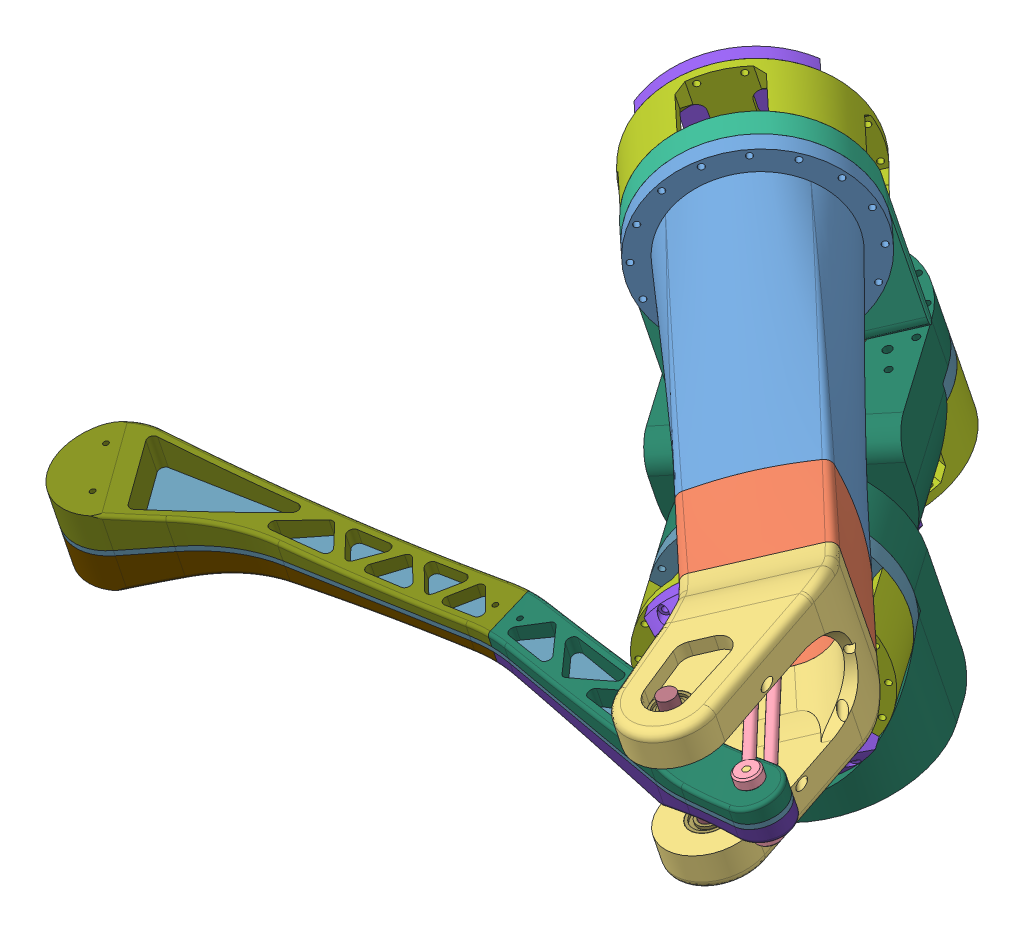
SolidWorks assembly Leg, configuration Default. Lengths in mm. (continued)
Components (placement in the parent): (continued)
- Cycloidal _v3-1: Cycloidal _v3 [Default] at (225.629 71.2826 236.7117) x (-0.201502 -0.265168 0.942912) z (-0.972255 -0.062625 -0.225384) size (173.36 87.57 173.15) (continued)
  - foc-motor-controller.step-1: foc-motor-controller.step [Default] at (47.4677 32.6574 89.6282) x (0.701413 0.00028 0.712755) z (0.000399 -1 0) size (57.23 50 8.13) (continued)
    - C_0603_1608Metric.step-24: C_0603_1608Metric.step [Default] at (-5.9 -16.6 1.595) x (0 1 0) z (0 0 1) size (1.6 0.8 0.8)
    - C_0603_1608Metric.step-25: C_0603_1608Metric.step [Default] at (-3.1 -14.1 1.595) size (1.6 0.8 0.8)
    - R_0603_1608Metric.step-21: R_0603_1608Metric.step [Default] at (7.2 -7.375 1.595) x (0 -1 0) z (0 0 1) size (1.6 0.8 0.45)
    - C_1206_3216Metric.step-15: C_1206_3216Metric.step [Default] at (-0.7 11 1.595) x (0 1 0) z (0 0 1) size (3.2 1.6 1.6)
    - LQFP-64_10x10mm_P0.5mm.step-1: LQFP-64_10x10mm_P0.5mm.step [Default] at (-7 -4.5 1.595) x (-1 0 0) z (0 0 1) size (12 12 1.5)
    - C_0805_2012Metric.step-2: C_0805_2012Metric.step [Default] at (23.35 -17 1.595) x (-1 0 0) z (0 0 1) size (2 1.25 1.25)
    - C_0603_1608Metric.step-26: C_0603_1608Metric.step [Default] at (10.8 -16.8 1.595) x (0 -1 0) z (0 0 1) size (1.6 0.8 0.8)
    - R_0603_1608Metric.step-22: R_0603_1608Metric.step [Default] at (17.5 -17.8 1.595) x (0 -1 0) z (0 0 1) size (1.6 0.8 0.45)
    - C_1206_3216Metric.step-16: C_1206_3216Metric.step [Default] at (20.3 11 1.595) x (0 1 0) z (0 0 1) size (3.2 1.6 1.6)
    - R_0603_1608Metric.step-23: R_0603_1608Metric.step [Default] at (9.2 -16.8 1.595) x (0 -1 0) z (0 0 1) size (1.6 0.8 0.45)
    - C_1206_3216Metric.step-17: C_1206_3216Metric.step [Default] at (-10 11 1.595) x (0 1 0) z (0 0 1) size (3.2 1.6 1.6)
    - R_0603_1608Metric.step-24: R_0603_1608Metric.step [Default] at (17.8 -15.2 1.595) size (1.6 0.8 0.45)
    - C_1206_3216Metric.step-18: C_1206_3216Metric.step [Default] at (19.9 2.6 1.595) x (-0.707107 0.707107 0) z (0 0 1) size (3.2 1.6 1.6)
    - C_0603_1608Metric.step-27: C_0603_1608Metric.step [Default] at (13.4 -7.375 1.595) x (0 -1 0) z (0 0 1) size (1.6 0.8 0.8)
    - R_0603_1608Metric.step-25: R_0603_1608Metric.step [Default] at (8.7 -7.375 1.595) x (0 -1 0) z (0 0 1) size (1.6 0.8 0.45)
    - PQFN-8-EP_6x5mm_P1.27mm_Generic.step-1: PQFN-8-EP_6x5mm_P1.27mm_Generic.step [Default] at (4.9 14.4 -0.085) x (0 1 0) z (0 0 -1) size (6.15 5.15 1.09)
    - C_0805_2012Metric.step-3: C_0805_2012Metric.step [Default] at (-3 8.9 -0.085) x (0 1 0) z (0 0 -1) size (2 1.25 1.25)
    - C_0603_1608Metric.step-28: C_0603_1608Metric.step [Default] at (1.5 -4.3 -0.085) x (0 1 0) z (0 0 -1) size (1.6 0.8 0.8)
    - R_2512_6332Metric.step-1: R_2512_6332Metric.step [Default] at (2.1 8.6 -0.085) x (-1 0 0) z (0 0 -1) size (6.3 3.2 0.6)
    - C_0805_2012Metric.step-4: C_0805_2012Metric.step [Default] at (18.8 8.9 -0.085) x (0 1 0) z (0 0 -1) size (2 1.25 1.25)
    - C_0805_2012Metric.step-5: C_0805_2012Metric.step [Default] at (-5.2 8.901 -0.085) x (0 1 0) z (0 0 -1) size (2 1.25 1.25)
    - PQFN-8-EP_6x5mm_P1.27mm_Generic.step-2: PQFN-8-EP_6x5mm_P1.27mm_Generic.step [Default] at (16.9 14.6 -0.085) x (0 -1 0) z (0 0 -1) size (6.15 5.15 1.09)
    - PQFN-8-EP_6x5mm_P1.27mm_Generic.step-3: PQFN-8-EP_6x5mm_P1.27mm_Generic.step [Default] at (-1.1 14.6 -0.085) x (0 -1 0) z (0 0 -1) size (6.15 5.15 1.09)
    - R_0603_1608Metric.step-26: R_0603_1608Metric.step [Default] at (8.2 8.8 -0.085) x (0 1 0) z (0 0 -1) size (1.6 0.8 0.45)
    - R_2512_6332Metric.step-2: R_2512_6332Metric.step [Default] at (-10.3 8.601 -0.085) x (1 0 0) z (0 0 -1) size (6.3 3.2 0.6)
    - TSSOP-16_4.4x5mm_P0.65mm.step-1: TSSOP-16_4.4x5mm_P0.65mm.step [Default] at (0 0 -0.085) x (-1 0 0) z (0 0 -1) size (6.4 5 1.1)
    - C_0603_1608Metric.step-29: C_0603_1608Metric.step [Default] at (0 -4.25 -0.085) x (0 1 0) z (0 0 -1) size (1.6 0.8 0.8)
    - PQFN-8-EP_6x5mm_P1.27mm_Generic.step-4: PQFN-8-EP_6x5mm_P1.27mm_Generic.step [Default] at (10.9 14.4 -0.085) x (0 1 0) z (0 0 -1) size (6.15 5.15 1.09)
    - R_2512_6332Metric.step-3: R_2512_6332Metric.step [Default] at (13.7 8.6 -0.085) x (1 0 0) z (0 0 -1) size (6.3 3.2 0.6)
    - PQFN-8-EP_6x5mm_P1.27mm_Generic.step-5: PQFN-8-EP_6x5mm_P1.27mm_Generic.step [Default] at (-13.1 14.401 -0.085) x (0 1 0) z (0 0 -1) size (6.15 5.15 1.09)
    - C_0603_1608Metric.step-30: C_0603_1608Metric.step [Default] at (-1.5 -4.3 -0.085) x (0 -1 0) z (0 0 -1) size (1.6 0.8 0.8)
    - PQFN-8-EP_6x5mm_P1.27mm_Generic.step-6: PQFN-8-EP_6x5mm_P1.27mm_Generic.step [Default] at (-7.1 14.601 -0.085) x (0 -1 0) z (0 0 -1) size (6.15 5.15 1.09)
    - foc-motor-controller_PCB.step-1: foc-motor-controller_PCB.step [Default] at origin size (50 50 1.51)
  - hex nut style 1 gradeab_iso-1: hex nut style 1 gradeab_iso [ISO - 4032 - M3 - W - N] at (47.7115 32.6575 59.2236) x (1 0.000399 0) z (0.000399 -1 0) size (5.5 6.35 2.4)
  - Cycloidal_Discs_8308-1: Cycloidal_Discs_8308 [Default] at (-11.9184 124.164 51.5043) x (0.028527 0.000011 0.999593) z (0.999593 0.000399 -0.028527) size (79.25 5 79.73)
    - Cycloidal_Discs-1: Cycloidal_Discs [Default] at (38.3081 39.5303 58.0959) size (79.25 5 79.73)
  - Cycloidal_Discs_8308-2: Cycloidal_Discs_8308 [Default] at (62.1667 47.133 159.1742) x (-0.931329 -0.000371 -0.364178) z (0.364178 0.000145 -0.931329) size (79.25 5 79.73)
    - Cycloidal_Discs-1: Cycloidal_Discs [Default] at (38.3081 39.5303 58.0959) size (79.25 5 79.73)
  - Motor_Cover_v2-2: Motor_Cover_v2 [Default] at (47.4667 35.0574 89.6282) x (0.999968 0.000399 0.00802) z (-0.00802 -0.000003 0.999968) size (115 34.6 115)
  - driver_cover-1: driver_cover [Default] at (47.4667 35.0574 89.6282) x (0.702656 0.00028 0.711529) z (0.711529 0.000284 -0.702656) size (81.32 15 115)
  - Cover_new-1: Cover_new [Default] at (47.4437 92.6574 89.6282) x (0.701413 0.00028 0.712755) z (-0.712755 -0.000284 0.701413) size (115 87.5 130)
  - Output_Shaft-2: Output_Shaft [Default] at (47.4437 92.6574 89.6282) x (0.572675 0.000228 0.819783) z (-0.819783 -0.000327 0.572675) size (70 14 70)
  - radial ball bearing_68_iso-47: radial ball bearing_68_iso [ISO 15 RBB - 289 - 14,SI,NC,14_68] at (61.9924 89.1632 109.081) x (0.000399 -1 0) z (-0.055662 -0.000022 0.99845) size (5 17 17)
  - radial ball bearing_68_iso-48: radial ball bearing_68_iso [ISO 15 RBB - 289 - 14,SI,NC,14_68] at (59.3269 82.1622 107.722) x (0.000399 -1 0) z (-0.055662 -0.000022 0.99845) size (5 17 17)
  - m4x14-1: m4x14 [Default] at (47.0925 68.4573 134.6267) x (0.999623 0.000399 0.027466) z (-0.027466 -0.000011 0.999623) size (8 15.2 8)
  - M3x20-1: M3x20 [Default] at (43.4726 96.3558 90.1203) x (-0.837193 -0.000334 -0.546908) z (-0.546908 -0.000218 0.837193) size (6 21.2 6)
  - M3x10-1: M3x10 [Default] at (36.5111 25.853 142.5044) x (0.424034 0.000169 -0.905646) z (0.905646 0.000361 0.424034) size (6 11.2 6)
  - m3x60-1: m3x60 [Default] at (17.1068 35.0453 134.2855) x (-0.837193 -0.000334 -0.546908) z (-0.546908 -0.000218 0.837193) size (5.3 63 5.3)
  - m6-1: m6 [Default] at (60.6129 98.6627 108.4832) x (-0.153131 -0.000061 0.988206) z (0.988206 0.000394 0.153131) size (6 16 6)
- Cycloidal _v3-2: Cycloidal _v3 [Default] at (146.1775 22.9675 470.2476) x (0.670066 -0.524344 -0.525427) z (0.511404 0.83914 -0.185227) size (173.36 87.57 173.15)
  - motor-X83008S.stp-1: motor-X83008S.stp [Default] at (3.9105 88.7742 94.1058) x (0.928336 0.00037 -0.371741) z (0.000399 -1 0) size (114.7 114.7 37.62) (hidden)
    - base.stp-1: base.stp [Default] at (42.0794 12.0269 46.7342) size (91.6 91.6 15.61)
    - stator.stp-1: stator.stp [Default] at (42.0794 12.0269 33.1342) x (0.08493 -0.996387 0) z (0 0 1) size (83 83 8)
    - coil.stp-1: coil.stp [Default] at (39.5332 41.8984 37.1342) x (0.996387 0.08493 0) z (-0.08493 0.996387 0) size (4.4 10.2 10.5)
    - coil.stp-2: coil.stp [Default] at (34.3848 41.0025 37.1342) x (0.966502 0.256661 0) z (-0.256661 0.966502 0) size (4.4 10.2 10.5)
    - coil.stp-3: coil.stp [Default] at (29.4701 39.2261 37.1342) x (0.90725 0.420593 0) z (-0.420593 0.90725 0) size (4.4 10.2 10.5)
    - coil.stp-4: coil.stp [Default] at (24.9386 36.6233 37.1342) x (0.820431 0.571745 0) z (-0.571745 0.820431 0) size (4.4 10.2 10.5)
    - coil.stp-5: coil.stp [Default] at (20.9279 33.2732 37.1342) x (0.708685 0.705525 0) z (-0.705525 0.708685 0) size (4.4 10.2 10.5)
    - coil.stp-6: coil.stp [Default] at (17.5599 29.2775 37.1342) x (0.575405 0.817869 0) z (-0.817869 0.575405 0) size (4.4 10.2 10.5)
    - coil.stp-7: coil.stp [Default] at (14.9368 24.7576 37.1342) x (0.424642 0.905361 0) z (-0.905361 0.424642 0) size (4.4 10.2 10.5)
    - coil.stp-8: coil.stp [Default] at (13.1385 19.8509 37.1342) x (0.260976 0.965345 0) z (-0.965345 0.260976 0) size (4.4 10.2 10.5)
    - coil.stp-9: coil.stp [Default] at (12.2196 14.7066 37.1342) x (0.089381 0.995998 0) z (-0.995998 0.089381 0) size (4.4 10.2 10.5)
    - coil.stp-10: coil.stp [Default] at (12.2079 9.4807 37.1342) x (-0.08493 0.996387 0) z (-0.996387 -0.08493 0) size (4.4 10.2 10.5)
    - coil.stp-11: coil.stp [Default] at (13.1039 4.3323 37.1342) x (-0.256661 0.966502 0) z (-0.966502 -0.256661 0) size (4.4 10.2 10.5)
    - coil.stp-12: coil.stp [Default] at (14.8802 -0.5824 37.1342) x (-0.420593 0.90725 0) z (-0.90725 -0.420593 0) size (4.4 10.2 10.5)
    - coil.stp-13: coil.stp [Default] at (17.483 -5.1139 37.1342) x (-0.571745 0.820431 0) z (-0.820431 -0.571745 0) size (4.4 10.2 10.5)
    - coil.stp-14: coil.stp [Default] at (20.8332 -9.1246 37.1342) x (-0.705525 0.708685 0) z (-0.708685 -0.705525 0) size (4.4 10.2 10.5)
    - coil.stp-15: coil.stp [Default] at (24.8289 -12.4926 37.1342) x (-0.817869 0.575405 0) z (-0.575405 -0.817869 0) size (4.4 10.2 10.5)
    - coil.stp-16: coil.stp [Default] at (29.3487 -15.1157 37.1342) x (-0.905361 0.424642 0) z (-0.424642 -0.905361 0) size (4.4 10.2 10.5)
    - coil.stp-17: coil.stp [Default] at (34.2554 -16.914 37.1342) x (-0.965345 0.260976 0) z (-0.260976 -0.965345 0) size (4.4 10.2 10.5)
    - coil.stp-18: coil.stp [Default] at (39.3998 -17.8329 37.1342) x (-0.995998 0.089381 0) z (-0.089381 -0.995998 0) size (4.4 10.2 10.5)
    - coil.stp-19: coil.stp [Default] at (44.6256 -17.8446 37.1342) x (-0.996387 -0.08493 0) z (0.08493 -0.996387 0) size (4.4 10.2 10.5)
    - coil.stp-20: coil.stp [Default] at (49.7741 -16.9486 37.1342) x (-0.966502 -0.256661 0) z (0.256661 -0.966502 0) size (4.4 10.2 10.5)
    - coil.stp-21: coil.stp [Default] at (54.6887 -15.1723 37.1342) x (-0.90725 -0.420593 0) z (0.420593 -0.90725 0) size (4.4 10.2 10.5)
    - coil.stp-22: coil.stp [Default] at (59.2202 -12.5695 37.1342) x (-0.820431 -0.571745 0) z (0.571745 -0.820431 0) size (4.4 10.2 10.5)
    - coil.stp-23: coil.stp [Default] at (63.2309 -9.2193 37.1342) x (-0.708685 -0.705525 0) z (0.705525 -0.708685 0) size (4.4 10.2 10.5)
    - coil.stp-24: coil.stp [Default] at (66.599 -5.2236 37.1342) x (-0.575405 -0.817869 0) z (0.817869 -0.575405 0) size (4.4 10.2 10.5)
    - coil.stp-25: coil.stp [Default] at (69.222 -0.7038 37.1342) x (-0.424642 -0.905361 0) z (0.905361 -0.424642 0) size (4.4 10.2 10.5)
    - coil.stp-26: coil.stp [Default] at (71.0203 4.2029 37.1342) x (-0.260976 -0.965345 0) z (0.965345 -0.260976 0) size (4.4 10.2 10.5)
    - coil.stp-27: coil.stp [Default] at (71.9392 9.3473 37.1342) x (-0.089381 -0.995998 0) z (0.995998 -0.089381 0) size (4.4 10.2 10.5)
    - coil.stp-28: coil.stp [Default] at (71.9509 14.5731 37.1342) x (0.08493 -0.996387 0) z (0.996387 0.08493 0) size (4.4 10.2 10.5)
    - coil.stp-29: coil.stp [Default] at (71.055 19.7216 37.1342) x (0.256661 -0.966502 0) z (0.966502 0.256661 0) size (4.4 10.2 10.5)
    - coil.stp-30: coil.stp [Default] at (69.2786 24.6362 37.1342) x (0.420593 -0.90725 0) z (0.90725 0.420593 0) size (4.4 10.2 10.5)
    - coil.stp-31: coil.stp [Default] at (66.6758 29.1677 37.1342) x (0.571745 -0.820431 0) z (0.820431 0.571745 0) size (4.4 10.2 10.5)
    - coil.stp-32: coil.stp [Default] at (63.3257 33.1785 37.1342) x (0.705525 -0.708685 0) z (0.708685 0.705525 0) size (4.4 10.2 10.5)
    - coil.stp-33: coil.stp [Default] at (59.33 36.5465 37.1342) x (0.817869 -0.575405 0) z (0.575405 0.817869 0) size (4.4 10.2 10.5)
    - coil.stp-34: coil.stp [Default] at (54.8101 39.1695 37.1342) x (0.905361 -0.424642 0) z (0.424642 0.905361 0) size (4.4 10.2 10.5)
    - coil.stp-35: coil.stp [Default] at (49.9034 40.9678 37.1342) x (0.965345 -0.260976 0) z (0.260976 0.965345 0) size (4.4 10.2 10.5)
    - coil.stp-36: coil.stp [Default] at (44.759 41.8868 37.1342) x (0.995998 -0.089381 0) z (0.089381 0.995998 0) size (4.4 10.2 10.5)
    - rotor.stp-1: rotor.stp [Default] at (42.0794 12.0269 42.1342) x (-0.293442 0.955977 0) z (0 0 -1) size (91.8 91.8 12)
    - outrunner.stp-1: outrunner.stp [Default] at (42.0794 12.0269 30.1342) x (-0.254711 0.967017 0) z (-0.967017 -0.254711 0) size (91.8 17.01 91.8)
    - screw-mount.stp-1: screw-mount.stp [Default] at (38.1314 27.0157 27.1342) x (1 0 0) z (0 0 -1) size (7 7 6.5)
    - screw-mount.stp-2: screw-mount.stp [Default] at (27.0906 8.0789 27.1342) x (1 0 0) z (0 0 -1) size (7 7 6.5)
    - screw-mount.stp-3: screw-mount.stp [Default] at (57.0682 15.9749 27.1342) x (1 0 0) z (0 0 -1) size (7 7 6.5)
    - screw-mount.stp-4: screw-mount.stp [Default] at (46.0274 -2.9618 27.1342) x (1 0 0) z (0 0 -1) size (7 7 6.5)
    - 6702ZZ-bearing-15x21x4.stp-1: 6702ZZ-bearing-15x21x4.stp [Default] at (42.0794 12.0269 43.7342) x (1 0 0) z (0 -1 0) size (21 4 21)
    - 6702ZZ-bearing-15x21x4.stp-2: 6702ZZ-bearing-15x21x4.stp [Default] at (42.0794 12.0269 35.1342) x (1 0 0) z (0 1 0) size (21 4 21)
    - shaft.stp-1: shaft.stp [Default] at (42.0794 12.0269 20.1342) size (16 16 31.6)
    - fix-screw.stp-1: fix-screw.stp [Default] at (42.0794 12.0269 51.7342) x (1 0 0) z (0 0 -1) size (19.67 18.96 12.02)
  - Base_Plate-1: Base_Plate [Default] at (47.4533 68.6574 89.6282) x (-0.992404 -0.000396 0.123023) z (-0.123023 -0.000049 -0.992404) size (39.8 11 39.8)
  - Eccentric_Shaft-1: Eccentric_Shaft [Default] at (60.4961 73.3217 80.3225) x (0.123023 0.000049 0.992404) z (-0.992404 -0.000396 0.123023) size (20 17 17)
    - Eccentric_Shaft_bot-1: Eccentric_Shaft_bot [Default] at (7.6302 12.3409 14.0904) x (1 0 0) z (0 0 -1) size (17 6 17)
    - Eccentric_Shaft_bot-2: Eccentric_Shaft_bot [Default] at (7.6302 12.3409 14.0904) x (-1 0 0) z (0 0 -1) size (17 6 17)
    - Eccentric_Shaft_top-1: Eccentric_Shaft_top [Default] at (7.6302 18.3409 14.0904) x (-1 0 0) z (0 0 -1) size (17 5 17)
  - radial ball bearing_68_iso-39: radial ball bearing_68_iso [ISO 15 RBB - 1860 - 32,SI,NC,32_68] at (47.4409 99.6574 89.6282) x (0.000399 -1 0) z (-0.546908 -0.000218 0.837193) size (10 78 78)
  - radial ball bearing_68_iso-40: radial ball bearing_68_iso [ISO 15 RBB - 1840 - 32,SI,NC,32_68] at (47.4516 72.9574 89.6282) x (-0.000399 1 0) z (0.001003 0 0.999999) size (7 52 52)
  - Base_plate_2-1: Base_plate_2 [Default] at (47.4529 69.6574 89.6282) x (0.712755 0.000284 -0.701413) z (0.701413 0.00028 0.712755) size (115 10 115)
  - m13_bearing-31: m13_bearing [Default] at (-10.4263 95.4017 67.196) x (0.227678 0.000091 0.973736) z (0.973736 0.000388 -0.227678) size (13 16 13)
    - m6-1: m6 [Default] at (8.4921 2.5508 14.8914) size (6 16 6)
    - radial ball bearing_68_iso-1: radial ball bearing_68_iso [ISO 15 RBB - 286 - 10,SI,NC,10_68] at (8.4921 16.0508 14.8914) x (0 1 0) z (0 0 1) size (5 13 13)
    - radial ball bearing_68_iso-2: radial ball bearing_68_iso [ISO 15 RBB - 286 - 10,SI,NC,10_68] at (8.4921 11.0508 14.8914) x (0 1 0) z (0 0 1) size (5 13 13)
  - m13_bearing-32: m13_bearing [Default] at (-13.9908 98.1837 84.3887) x (0.227678 0.000091 0.973736) z (0.973736 0.000388 -0.227678) size (13 16 13)
    - m6-1: m6 [Default] at (8.4921 2.5508 14.8914) size (6 16 6)
    - radial ball bearing_68_iso-1: radial ball bearing_68_iso [ISO 15 RBB - 286 - 10,SI,NC,10_68] at (8.4921 16.0508 14.8914) x (0 1 0) z (0 0 1) size (5 13 13)
    - radial ball bearing_68_iso-2: radial ball bearing_68_iso [ISO 15 RBB - 286 - 10,SI,NC,10_68] at (8.4921 11.0508 14.8914) x (0 1 0) z (0 0 1) size (5 13 13)
  - m13_bearing-34: m13_bearing [Default] at (13.4541 98.1947 126.1847) x (0.227678 0.000091 0.973736) z (0.973736 0.000388 -0.227678) size (13 16 13)
    - m6-1: m6 [Default] at (8.4921 2.5508 14.8914) size (6 16 6)
    - radial ball bearing_68_iso-1: radial ball bearing_68_iso [ISO 15 RBB - 286 - 10,SI,NC,10_68] at (8.4921 16.0508 14.8914) x (0 1 0) z (0 0 1) size (5 13 13)
    - radial ball bearing_68_iso-2: radial ball bearing_68_iso [ISO 15 RBB - 286 - 10,SI,NC,10_68] at (8.4921 11.0508 14.8914) x (0 1 0) z (0 0 1) size (5 13 13)
  - m13_bearing-35: m13_bearing [Default] at (-1.0662 98.1889 116.3132) x (0.227678 0.000091 0.973736) z (0.973736 0.000388 -0.227678) size (13 16 13)
    - m6-1: m6 [Default] at (8.4921 2.5508 14.8914) size (6 16 6)
    - radial ball bearing_68_iso-1: radial ball bearing_68_iso [ISO 15 RBB - 286 - 10,SI,NC,10_68] at (8.4921 16.0508 14.8914) x (0 1 0) z (0 0 1) size (5 13 13)
    - radial ball bearing_68_iso-2: radial ball bearing_68_iso [ISO 15 RBB - 286 - 10,SI,NC,10_68] at (8.4921 11.0508 14.8914) x (0 1 0) z (0 0 1) size (5 13 13)
  - m13_bearing-36: m13_bearing [Default] at (-10.7036 98.185 101.6364) x (0.227678 0.000091 0.973736) z (0.973736 0.000388 -0.227678) size (13 16 13)
    - m6-1: m6 [Default] at (8.4921 2.5508 14.8914) size (6 16 6)
    - radial ball bearing_68_iso-1: radial ball bearing_68_iso [ISO 15 RBB - 286 - 10,SI,NC,10_68] at (8.4921 16.0508 14.8914) x (0 1 0) z (0 0 1) size (5 13 13)
    - radial ball bearing_68_iso-2: radial ball bearing_68_iso [ISO 15 RBB - 286 - 10,SI,NC,10_68] at (8.4921 11.0508 14.8914) x (0 1 0) z (0 0 1) size (5 13 13)
  - m13_bearing-1: m13_bearing [Default] at (-0.4494 98.1891 62.778) x (0.736525 0.000294 0.676411) z (0.676411 0.00027 -0.736525) size (13 16 13)
    - m6-1: m6 [Default] at (8.4921 2.5508 14.8914) size (6 16 6)
    - radial ball bearing_68_iso-1: radial ball bearing_68_iso [ISO 15 RBB - 286 - 10,SI,NC,10_68] at (8.4921 16.0508 14.8914) x (0 1 0) z (0 0 1) size (5 13 13)
    - radial ball bearing_68_iso-2: radial ball bearing_68_iso [ISO 15 RBB - 286 - 10,SI,NC,10_68] at (8.4921 11.0508 14.8914) x (0 1 0) z (0 0 1) size (5 13 13)
  - m13_bearing-2: m13_bearing [Default] at (48.5236 98.2087 124.7001) x (0.120271 0.000048 0.992741) z (0.992741 0.000396 -0.120271) size (13 16 13)
    - m6-1: m6 [Default] at (8.4921 2.5508 14.8914) size (6 16 6)
    - radial ball bearing_68_iso-1: radial ball bearing_68_iso [ISO 15 RBB - 286 - 10,SI,NC,10_68] at (8.4921 16.0508 14.8914) x (0 1 0) z (0 0 1) size (5 13 13)
    - radial ball bearing_68_iso-2: radial ball bearing_68_iso [ISO 15 RBB - 286 - 10,SI,NC,10_68] at (8.4921 11.0508 14.8914) x (0 1 0) z (0 0 1) size (5 13 13)
  - m13_bearing-3: m13_bearing [Default] at (32.5019 98.2023 52.3604) x (0.833889 0.000333 0.551933) z (0.551932 0.00022 -0.833889) size (13 16 13)
    - m6-1: m6 [Default] at (8.4921 2.5508 14.8914) size (6 16 6)
    - radial ball bearing_68_iso-1: radial ball bearing_68_iso [ISO 15 RBB - 286 - 10,SI,NC,10_68] at (8.4921 16.0508 14.8914) x (0 1 0) z (0 0 1) size (5 13 13)
    - radial ball bearing_68_iso-2: radial ball bearing_68_iso [ISO 15 RBB - 286 - 10,SI,NC,10_68] at (8.4921 11.0508 14.8914) x (0 1 0) z (0 0 1) size (5 13 13)
  - m13_bearing-4: m13_bearing [Default] at (77.3632 98.2202 81.8307) x (0.022268 0.000009 0.999752) z (0.999752 0.000399 -0.022268) size (13 16 13)
    - m6-1: m6 [Default] at (8.4921 2.5508 14.8914) size (6 16 6)
    - radial ball bearing_68_iso-1: radial ball bearing_68_iso [ISO 15 RBB - 286 - 10,SI,NC,10_68] at (8.4921 16.0508 14.8914) x (0 1 0) z (0 0 1) size (5 13 13)
    - radial ball bearing_68_iso-2: radial ball bearing_68_iso [ISO 15 RBB - 286 - 10,SI,NC,10_68] at (8.4921 11.0508 14.8914) x (0 1 0) z (0 0 1) size (5 13 13)
  - m13_bearing-5: m13_bearing [Default] at (73.5091 98.2186 99.5852) x (0.059133 0.000024 0.99825) z (0.99825 0.000398 -0.059133) size (13 16 13)
    - m6-1: m6 [Default] at (8.4921 2.5508 14.8914) size (6 16 6)
    - radial ball bearing_68_iso-1: radial ball bearing_68_iso [ISO 15 RBB - 286 - 10,SI,NC,10_68] at (8.4921 16.0508 14.8914) x (0 1 0) z (0 0 1) size (5 13 13)
    - radial ball bearing_68_iso-2: radial ball bearing_68_iso [ISO 15 RBB - 286 - 10,SI,NC,10_68] at (8.4921 11.0508 14.8914) x (0 1 0) z (0 0 1) size (5 13 13)
  - m13_bearing-6: m13_bearing [Default] at (13.4333 98.1947 47.0643) x (0.451561 0.00018 0.89224) z (0.89224 0.000356 -0.451561) size (13 16 13)
    - m6-1: m6 [Default] at (8.4921 2.5508 14.8914) size (6 16 6)
    - radial ball bearing_68_iso-1: radial ball bearing_68_iso [ISO 15 RBB - 286 - 10,SI,NC,10_68] at (8.4921 16.0508 14.8914) x (0 1 0) z (0 0 1) size (5 13 13)
    - radial ball bearing_68_iso-2: radial ball bearing_68_iso [ISO 15 RBB - 286 - 10,SI,NC,10_68] at (8.4921 11.0508 14.8914) x (0 1 0) z (0 0 1) size (5 13 13)
  - m13_bearing-7: m13_bearing [Default] at (57.1526 98.2121 32.9496) x (-0.545813 -0.000218 0.837907) z (0.837907 0.000334 0.545813) size (13 16 13)
    - m6-1: m6 [Default] at (8.4921 2.5508 14.8914) size (6 16 6)
    - radial ball bearing_68_iso-1: radial ball bearing_68_iso [ISO 15 RBB - 286 - 10,SI,NC,10_68] at (8.4921 16.0508 14.8914) x (0 1 0) z (0 0 1) size (5 13 13)
    - radial ball bearing_68_iso-2: radial ball bearing_68_iso [ISO 15 RBB - 286 - 10,SI,NC,10_68] at (8.4921 11.0508 14.8914) x (0 1 0) z (0 0 1) size (5 13 13)
  - m13_bearing-8: m13_bearing [Default] at (73.1034 98.2185 66.7178) x (0.158553 0.000063 0.98735) z (0.98735 0.000394 -0.158553) size (13 16 13)
    - m6-1: m6 [Default] at (8.4921 2.5508 14.8914) size (6 16 6)
    - radial ball bearing_68_iso-1: radial ball bearing_68_iso [ISO 15 RBB - 286 - 10,SI,NC,10_68] at (8.4921 16.0508 14.8914) x (0 1 0) z (0 0 1) size (5 13 13)
    - radial ball bearing_68_iso-2: radial ball bearing_68_iso [ISO 15 RBB - 286 - 10,SI,NC,10_68] at (8.4921 11.0508 14.8914) x (0 1 0) z (0 0 1) size (5 13 13)
  - m13_bearing-9: m13_bearing [Default] at (74.5316 98.219 41.6624) x (-0.687134 -0.000274 0.72653) z (0.72653 0.00029 0.687134) size (13 16 13)
    - m6-1: m6 [Default] at (8.4921 2.5508 14.8914) size (6 16 6)
    - radial ball bearing_68_iso-1: radial ball bearing_68_iso [ISO 15 RBB - 286 - 10,SI,NC,10_68] at (8.4921 16.0508 14.8914) x (0 1 0) z (0 0 1) size (5 13 13)
    - radial ball bearing_68_iso-2: radial ball bearing_68_iso [ISO 15 RBB - 286 - 10,SI,NC,10_68] at (8.4921 11.0508 14.8914) x (0 1 0) z (0 0 1) size (5 13 13)
  - m13_bearing-11: m13_bearing [Default] at (30.0113 98.2013 136.2104) x (0.57351 0.000229 0.819198) z (0.819198 0.000327 -0.57351) size (13 16 13)
    - m6-1: m6 [Default] at (8.4921 2.5508 14.8914) size (6 16 6)
    - radial ball bearing_68_iso-1: radial ball bearing_68_iso [ISO 15 RBB - 286 - 10,SI,NC,10_68] at (8.4921 16.0508 14.8914) x (0 1 0) z (0 0 1) size (5 13 13)
    - radial ball bearing_68_iso-2: radial ball bearing_68_iso [ISO 15 RBB - 286 - 10,SI,NC,10_68] at (8.4921 11.0508 14.8914) x (0 1 0) z (0 0 1) size (5 13 13)
  - m13_bearing-12: m13_bearing [Default] at (62.5932 98.2143 116.7506) x (0.22335 0.000089 0.974738) z (0.974738 0.000389 -0.22335) size (13 16 13)
    - m6-1: m6 [Default] at (8.4921 2.5508 14.8914) size (6 16 6)
    - radial ball bearing_68_iso-1: radial ball bearing_68_iso [ISO 15 RBB - 286 - 10,SI,NC,10_68] at (8.4921 16.0508 14.8914) x (0 1 0) z (0 0 1) size (5 13 13)
    - radial ball bearing_68_iso-2: radial ball bearing_68_iso [ISO 15 RBB - 286 - 10,SI,NC,10_68] at (8.4921 11.0508 14.8914) x (0 1 0) z (0 0 1) size (5 13 13)
  - M3x4x4.2_brass_insert-22: M3x4x4.2_brass_insert [Default] at (43.4837 68.6558 90.1203) x (0.984609 0.000393 -0.174769) z (0.174769 0.00007 0.984609) size (4 4 4)
  - M3x4x4.2_brass_insert-23: M3x4x4.2_brass_insert [Default] at (51.4229 68.659 89.1361) x (0.984609 0.000393 -0.174769) z (0.174769 0.00007 0.984609) size (4 4 4)
  - radial ball bearing_68_iso-44: radial ball bearing_68_iso [ISO 15 RBB - 1715 - 26,SI,NC,26_68] at (47.2636 81.6573 88.1396) x (0.000399 -1 0) z (0.171535 0.000068 0.985178) size (4 21 21)
  - radial ball bearing_68_iso-45: radial ball bearing_68_iso [ISO 15 RBB - 1715 - 26,SI,NC,26_68] at (47.4429 94.6574 89.6282) x (0.000399 -1 0) z (0.819169 0.000327 0.573552) size (4 21 21)
  - radial ball bearing_68_iso-46: radial ball bearing_68_iso [ISO 15 RBB - 1715 - 26,SI,NC,26_68] at (47.6295 89.6575 91.1168) x (-0.000399 1 0) z (0 0 1) size (4 21 21)
  - foc-motor-controller.step-1: foc-motor-controller.step [Default] at (47.4677 32.6574 89.6282) x (0.701413 0.00028 0.712755) z (0.000399 -1 0) size (57.23 50 8.13)
    - RTA0040B.step-1: RTA0040B.step [Default] at (12.5014 -1.6986 1.595) x (-0.707107 -0.707107 0) z (0 0 1) size (6 6 1)
      - FRAME.step-1: FRAME.step [Default] x (1 0 0) z (0 -1 0) size (6 0.2 6)
        - SOLID.step-1: SOLID.step [Default] at origin size (0.4 0.2 0.22)
        - SOLID-0.step-1: SOLID-0.step [Default] at origin size (0.4 0.2 0.22)
        - SOLID-1.step-1: SOLID-1.step [Default] at origin size (0.4 0.2 0.22)
        - SOLID-2.step-1: SOLID-2.step [Default] at origin size (0.4 0.2 0.22)
        - SOLID-3.step-1: SOLID-3.step [Default] at origin size (0.4 0.2 0.22)
        - SOLID-4.step-1: SOLID-4.step [Default] at origin size (0.4 0.2 0.22)
        - SOLID-5.step-1: SOLID-5.step [Default] at origin size (0.4 0.2 0.22)
        - SOLID-6.step-1: SOLID-6.step [Default] at origin size (0.4 0.2 0.22)
        - SOLID-7.step-1: SOLID-7.step [Default] at origin size (0.4 0.2 0.22)
        - SOLID-8.step-1: SOLID-8.step [Default] at origin size (0.4 0.2 0.22)
        - SOLID-9.step-1: SOLID-9.step [Default] at origin size (0.22 0.2 0.4)
        - SOLID-10.step-1: SOLID-10.step [Default] at origin size (0.22 0.2 0.4)
        - SOLID-11.step-1: SOLID-11.step [Default] at origin size (0.22 0.2 0.4)
        - SOLID-12.step-1: SOLID-12.step [Default] at origin size (0.22 0.2 0.4)
        - SOLID-13.step-1: SOLID-13.step [Default] at origin size (0.22 0.2 0.4)
        - SOLID-14.step-1: SOLID-14.step [Default] at origin size (0.22 0.2 0.4)
        - SOLID-15.step-1: SOLID-15.step [Default] at origin size (0.22 0.2 0.4)
        - SOLID-16.step-1: SOLID-16.step [Default] at origin size (0.22 0.2 0.4)
        - SOLID-17.step-1: SOLID-17.step [Default] at origin size (4.15 0.2 4.15)
        - SOLID-18.step-1: SOLID-18.step [Default] at origin size (0.28 0.1 0.28)
        - SOLID-19.step-1: SOLID-19.step [Default] at origin size (0.28 0.1 0.28)
        - SOLID-20.step-1: SOLID-20.step [Default] at origin size (0.28 0.1 0.28)
        - SOLID-21.step-1: SOLID-21.step [Default] at origin size (0.28 0.1 0.28)
        - SOLID-22.step-1: SOLID-22.step [Default] at origin size (0.4 0.2 0.22)
        - SOLID-23.step-1: SOLID-23.step [Default] at origin size (0.4 0.2 0.22)
        - SOLID-24.step-1: SOLID-24.step [Default] at origin size (0.4 0.2 0.22)
        - SOLID-25.step-1: SOLID-25.step [Default] at origin size (0.4 0.2 0.22)
        - SOLID-26.step-1: SOLID-26.step [Default] at origin size (0.4 0.2 0.22)
        - SOLID-27.step-1: SOLID-27.step [Default] at origin size (0.4 0.2 0.22)
        - SOLID-28.step-1: SOLID-28.step [Default] at origin size (0.4 0.2 0.22)
        - SOLID-29.step-1: SOLID-29.step [Default] at origin size (0.4 0.2 0.22)
        - SOLID-30.step-1: SOLID-30.step [Default] at origin size (0.4 0.2 0.22)
        - SOLID-31.step-1: SOLID-31.step [Default] at origin size (0.4 0.2 0.22)
        - SOLID-32.step-1: SOLID-32.step [Default] at origin size (0.22 0.2 0.4)
        - SOLID-33.step-1: SOLID-33.step [Default] at origin size (0.22 0.2 0.4)
        - SOLID-34.step-1: SOLID-34.step [Default] at origin size (0.22 0.2 0.4)
        - SOLID-35.step-1: SOLID-35.step [Default] at origin size (0.22 0.2 0.4)
        - SOLID-36.step-1: SOLID-36.step [Default] at origin size (0.22 0.2 0.4)
        - SOLID-37.step-1: SOLID-37.step [Default] at origin size (0.22 0.2 0.4)
        - SOLID-38.step-1: SOLID-38.step [Default] at origin size (0.22 0.2 0.4)
        - SOLID-39.step-1: SOLID-39.step [Default] at origin size (0.22 0.2 0.4)
        - SOLID-40.step-1: SOLID-40.step [Default] at origin size (0.22 0.2 0.4)
        - SOLID-41.step-1: SOLID-41.step [Default] at origin size (0.22 0.2 0.4)
        - SOLID-42.step-1: SOLID-42.step [Default] at origin size (0.22 0.2 0.4)
        - SOLID-43.step-1: SOLID-43.step [Default] at origin size (0.22 0.2 0.4)
      - BODY.step-1: BODY.step [Default] at (0 0 0.025) x (1 0 0) z (0 -1 0) size (6 0.97 6)
    - Resonator_SMD_Murata_CSTxExxV-3Pin_3.0x1.1mm.step-1: Resonator_SMD_Murata_CSTxExxV-3Pin_3.0x1.1mm.step [Default] at (1.8 -7 1.595) x (0 1 0) z (0 0 1) size (3.2 1.35 0.9)
    - C_0603_1608Metric.step-1: C_0603_1608Metric.step [Default] at (6.2 -16.8 1.595) x (0 -1 0) z (0 0 1) size (1.6 0.8 0.8)
    - R_0603_1608Metric.step-1: R_0603_1608Metric.step [Default] at (11.8 -7.375 1.595) x (0 1 0) z (0 0 1) size (1.6 0.8 0.45)
    - R_0603_1608Metric.step-2: R_0603_1608Metric.step [Default] at (13.8 -16.8 1.595) x (0 1 0) z (0 0 1) size (1.6 0.8 0.45)
    - R_0603_1608Metric.step-3: R_0603_1608Metric.step [Default] at (18.1 -5.36 1.595) size (1.6 0.8 0.45)
    - C_0603_1608Metric.step-2: C_0603_1608Metric.step [Default] at (2.6 -0.5 1.595) x (0 -1 0) z (0 0 1) size (1.6 0.8 0.8)
    - R_0603_1608Metric.step-4: R_0603_1608Metric.step [Default] at (14.6 -11.3 1.595) x (0 1 0) z (0 0 1) size (1.6 0.8 0.45)
    - L_APV_ANR4020.step-1: L_APV_ANR4020.step [Default] at (22.3 -13.7 1.595) x (0 -1 0) z (0 0 1) size (4.02 4 2)
    - C_0603_1608Metric.step-3: C_0603_1608Metric.step [Default] at (0.3 -12.6 1.595) x (-1 0 0) z (0 0 1) size (1.6 0.8 0.8)
    - C_1206_3216Metric.step-1: C_1206_3216Metric.step [Default] at (15.7 11 1.595) x (0 1 0) z (0 0 1) size (3.2 1.6 1.6)
    - C_0603_1608Metric.step-4: C_0603_1608Metric.step [Default] at (0.3 -9.6 1.595) size (1.6 0.8 0.8)
    - R_0603_1608Metric.step-5: R_0603_1608Metric.step [Default] at (12.3 -16.8 1.595) x (0 1 0) z (0 0 1) size (1.6 0.8 0.45)
    - C_0603_1608Metric.step-5: C_0603_1608Metric.step [Default] at (-0.3 -16.6 1.595) x (0 1 0) z (0 0 1) size (1.6 0.8 0.8)
    - R_0603_1608Metric.step-6: R_0603_1608Metric.step [Default] at (10.9 4.1 1.595) size (1.6 0.8 0.45)
    - C_1206_3216Metric.step-2: C_1206_3216Metric.step [Default] at (6.3 11 1.595) x (0 1 0) z (0 0 1) size (3.2 1.6 1.6)
    - XT30PW_2_2_-M.G.B.step-1: XT30PW_2_2_-M.G.B.step [Default] at (-20.5 9.5 1.595) x (0 -1 0) z (-1 0 0) size (15.5 7.1 12.53)
    - R_0603_1608Metric.step-7: R_0603_1608Metric.step [Default] at (0.3 -11.1 1.595) size (1.6 0.8 0.45)
    - C_0603_1608Metric.step-6: C_0603_1608Metric.step [Default] at (19 -0.4 1.595) x (-0.707107 -0.707107 0) z (0 0 1) size (1.6 0.8 0.8)
    - C_1206_3216Metric.step-3: C_1206_3216Metric.step [Default] at (13.3 11 1.595) x (0 1 0) z (0 0 1) size (3.2 1.6 1.6)
    - R_0603_1608Metric.step-8: R_0603_1608Metric.step [Default] at (10.2 -7.375 1.595) x (0 -1 0) z (0 0 1) size (1.6 0.8 0.45)
    - JST_GH_SM08B-GHS-TB_1x08-1MP_P1.25mm_Horizontal.step-1: JST_GH_SM08B-GHS-TB_1x08-1MP_P1.25mm_Horizontal.step [Default] at (10 -22 1.595) size (13.25 4.95 4.25)
    - C_1206_3216Metric.step-4: C_1206_3216Metric.step [Default] at (-12.3 11 1.595) x (0 1 0) z (0 0 1) size (3.2 1.6 1.6)
    - JST_GH_SM06B-GHS-TB_1x06-1MP_P1.25mm_Horizontal.step-1: JST_GH_SM06B-GHS-TB_1x06-1MP_P1.25mm_Horizontal.step [Default] at (-4.3 -22 1.595) size (10.75 4.95 4.25)
    - C_0603_1608Metric.step-7: C_0603_1608Metric.step [Default] at (7.3 -4.5 1.595) x (-1 0 0) z (0 0 1) size (1.6 0.8 0.8)
    - R_0603_1608Metric.step-9: R_0603_1608Metric.step [Default] at (18.1 -3.86 1.595) x (-1 0 0) z (0 0 1) size (1.6 0.8 0.45)
    - C_1206_3216Metric.step-5: C_1206_3216Metric.step [Default] at (22.6794 -1.2206 1.595) x (0.707107 -0.707107 0) z (0 0 1) size (3.2 1.6 1.6)
    - R_Array_Convex_4x0402.step-1: R_Array_Convex_4x0402.step [Default] at (6.8 -2.5 1.595) size (1 2 0.35)
    - R_0603_1608Metric.step-10: R_0603_1608Metric.step [Default] at (7.7 -16.8 1.595) x (0 -1 0) z (0 0 1) size (1.6 0.8 0.45)
    - C_1206_3216Metric.step-6: C_1206_3216Metric.step [Default] at (8.7 11 1.595) x (0 1 0) z (0 0 1) size (3.2 1.6 1.6)
    - C_0603_1608Metric.step-8: C_0603_1608Metric.step [Default] at (16.1 -11.3 1.595) x (0 1 0) z (0 0 1) size (1.6 0.8 0.8)
    - SOT-23-5.step-1: SOT-23-5.step [Default] at (-3.1 -16.6 1.595) x (-1 0 0) z (0 0 1) size (2.8 2.9 1.55)
    - C_0603_1608Metric.step-9: C_0603_1608Metric.step [Default] at (17.8 -13.6 1.595) size (1.6 0.8 0.8)
    - R_0603_1608Metric.step-11: R_0603_1608Metric.step [Default] at (-11.5 -20.3875 1.595) x (0 -1 0) z (0 0 1) size (1.6 0.8 0.45)
    - C_0603_1608Metric.step-10: C_0603_1608Metric.step [Default] at (-12.4 2.3 1.595) x (0 1 0) z (0 0 1) size (1.6 0.8 0.8)
    - C_1206_3216Metric.step-7: C_1206_3216Metric.step [Default] at (18 11 1.595) x (0 1 0) z (0 0 1) size (3.2 1.6 1.6)
    - R_0603_1608Metric.step-12: R_0603_1608Metric.step [Default] at (-10.8105 -14.9971 1.595) x (-1 0 0) z (0 0 1) size (1.6 0.8 0.45)
    - C_0603_1608Metric.step-11: C_0603_1608Metric.step [Default] at (-13.8 -9.4 1.595) x (-1 0 0) z (0 0 1) size (1.6 0.8 0.8)
    - R_0603_1608Metric.step-13: R_0603_1608Metric.step [Default] at (-23.15 -14.5 1.595) x (-1 0 0) z (0 0 1) size (1.6 0.8 0.45)
    - C_0603_1608Metric.step-12: C_0603_1608Metric.step [Default] at (1.1 -0.2 1.595) x (0 1 0) z (0 0 1) size (1.6 0.8 0.8)
    - D_0805_2012Metric.step-1: D_0805_2012Metric.step [Default] at (22.9 -9.6 1.595) x (0 1 0) z (0 0 1) size (2 1.27 0.8)
    - C_0603_1608Metric.step-13: C_0603_1608Metric.step [Default] at (-7.8 3.775 1.595) x (0 -1 0) z (0 0 1) size (1.6 0.8 0.8)
    - R_0603_1608Metric.step-14: R_0603_1608Metric.step [Default] at (-6.4 -12.825 1.595) x (0 1 0) z (0 0 1) size (1.6 0.8 0.45)
    - L_0603_1608Metric.step-1: L_0603_1608Metric.step [Default] at (-10.1 3 1.595) size (1.6 0.8 0.8)
    - C_0603_1608Metric.step-14: C_0603_1608Metric.step [Default] at (17.9 0.7 1.595) x (-0.707107 -0.707107 0) z (0 0 1) size (1.6 0.8 0.8)
    - HVSSOP-10.step-1: HVSSOP-10.step [Default] at (18.6 -9.6 1.595) x (0 -1 0) z (-1 0 0) size (4.9 1.1 3)
    - C_0603_1608Metric.step-15: C_0603_1608Metric.step [Default] at (7.9 4.1 1.595) x (-1 0 0) z (0 0 1) size (1.6 0.8 0.8)
    - C_0603_1608Metric.step-16: C_0603_1608Metric.step [Default] at (21.1 -9.6 1.595) x (0 -1 0) z (0 0 1) size (1.6 0.8 0.8)
    - R_0603_1608Metric.step-15: R_0603_1608Metric.step [Default] at (-10.8105 -11.9971 1.595) x (-1 0 0) z (0 0 1) size (1.6 0.8 0.45)
    - R_0603_1608Metric.step-16: R_0603_1608Metric.step [Default] at (-18.2 -17.4 1.595) size (1.6 0.8 0.45)
    - C_1206_3216Metric.step-8: C_1206_3216Metric.step [Default] at (-3 11 1.595) x (0 1 0) z (0 0 1) size (3.2 1.6 1.6)
    - R_0603_1608Metric.step-17: R_0603_1608Metric.step [Default] at (-16.9 -20.4 1.595) x (0 -1 0) z (0 0 1) size (1.6 0.8 0.45)
    - R_0603_1608Metric.step-18: R_0603_1608Metric.step [Default] at (-13.3 -20.3875 1.595) x (0 -1 0) z (0 0 1) size (1.6 0.8 0.45)
    - R_0603_1608Metric.step-19: R_0603_1608Metric.step [Default] at (-15.1 -20.3875 1.595) x (0 -1 0) z (0 0 1) size (1.6 0.8 0.45)
    - C_0603_1608Metric.step-17: C_0603_1608Metric.step [Default] at (15.5 -14.4 1.595) x (0 -1 0) z (0 0 1) size (1.6 0.8 0.8)
    - LED_0603_1608Metric.step-1: LED_0603_1608Metric.step [Default] at (-11.5 -23.3875 1.595) x (0 1 0) z (0 0 1) size (1.6 0.8 1.1)
    - C_0805_2012Metric.step-1: C_0805_2012Metric.step [Default] at (19.95 -17 1.595) size (2 1.25 1.25)
    - D_SMB.step-1: D_SMB.step [Default] at (-16.5 11.208 1.595) x (0 -1 0) z (0 0 1) size (5.3 3.55 2.15)
    - C_1206_3216Metric.step-9: C_1206_3216Metric.step [Default] at (-5.3 11 1.595) x (0 1 0) z (0 0 1) size (3.2 1.6 1.6)
    - XT30PW_2_2_-M.G.B.step-2: XT30PW_2_2_-M.G.B.step [Default] at (-20.5 -6.5 1.595) x (0 -1 0) z (-1 0 0) size (15.5 7.1 12.53)
    - C_1206_3216Metric.step-10: C_1206_3216Metric.step [Default] at (1.7 11 1.595) x (0 1 0) z (0 0 1) size (3.2 1.6 1.6)
    - C_1206_3216Metric.step-11: C_1206_3216Metric.step [Default] at (11 11 1.595) x (0 1 0) z (0 0 1) size (3.2 1.6 1.6)
    - C_0603_1608Metric.step-18: C_0603_1608Metric.step [Default] at (-6.3 3.775 1.595) x (0 -1 0) z (0 0 1) size (1.6 0.8 0.8)
    - C_0603_1608Metric.step-19: C_0603_1608Metric.step [Default] at (16.8686 1.7314 1.595) x (0.707107 0.707107 0) z (0 0 1) size (1.6 0.8 0.8)
    - C_0603_1608Metric.step-20: C_0603_1608Metric.step [Default] at (-15.0105 -11.1 1.595) size (1.6 0.8 0.8)
    - C_1206_3216Metric.step-12: C_1206_3216Metric.step [Default] at (-7.7 11 1.595) x (0 1 0) z (0 0 1) size (3.2 1.6 1.6)
    - C_0603_1608Metric.step-21: C_0603_1608Metric.step [Default] at (-18.2 -15.8 1.595) size (1.6 0.8 0.8)
    - C_0603_1608Metric.step-22: C_0603_1608Metric.step [Default] at (-2.1 -11.3 1.595) x (0 -1 0) z (0 0 1) size (1.6 0.8 0.8)
    - C_0603_1608Metric.step-23: C_0603_1608Metric.step [Default] at (-10.8105 -13.4971 1.595) size (1.6 0.8 0.8)
